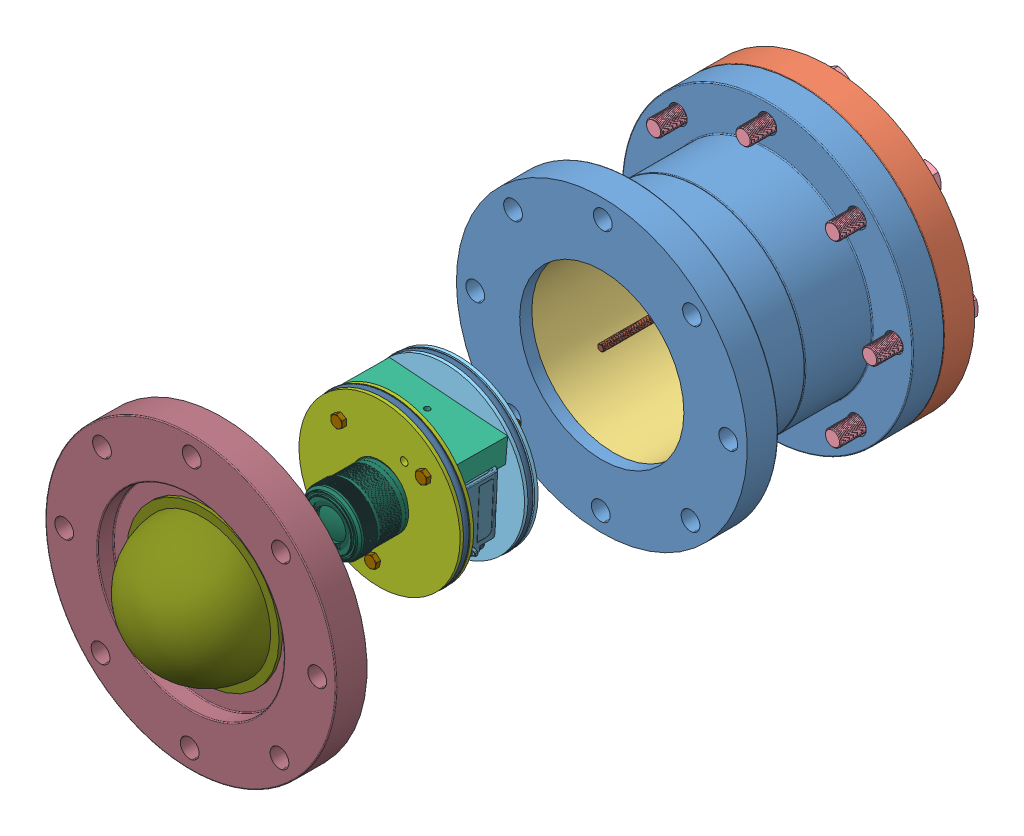
SolidWorks assembly Photogrametry_V5-PVC - exploded, configuration Default. Lengths in mm.
Overall size (484.92 484.92 825.6).
31 component instances, 16 part files, 0 mates.
Components (placement in the parent):
- externalHousing-Assembly-1: externalHousing-Assembly [Default] at (41.8532 87.3209 72.2129) size (484.92 484.92 280.15)
  - 8in PVC Flange-1: 8in PVC Flange [4881K224] at (120.5656 188.2131 202.8846) size (342.9 342.9 115.89)
  - 8in PVC Flange Closed-1: 8in PVC Flange Closed [4881K973] at (120.5656 188.2131 166.3721) size (342.9 342.9 36.51)
  - 8in PVC Pipe-1: 8in PVC Pipe [48855K43] at (120.5656 188.2131 318.8302) x (0.914978 0.403503 0) z (0 0 1) size (219.07 219.07 203.2)
  - 8in PVC Flange-2: 8in PVC Flange [4881K224] at (120.5656 188.2131 434.6169) x (-0.71277 -0.701398 0) z (0 0 -1) size (342.9 342.9 115.89)
  - BOLT 3-4in x 4in-1: BOLT 3-4in x 4in [92198A390] at (120.5656 337.4381 211.219) x (0 0 1) z (-0.999812 -0.019405 0) size (114.21 33 28.57)
  - BOLT 3-4in x 4in-2: BOLT 3-4in x 4in [92198A390] at (120.5656 38.9881 211.219) x (0 0 1) z (-0.865453 -0.50099 0) size (114.21 33 28.57)
  - BOLT 3-4in x 4in-3: BOLT 3-4in x 4in [92198A390] at (269.7906 188.2131 211.219) x (0 0 1) z (-0.997964 -0.063786 0) size (114.21 33 28.57)
  - BOLT 3-4in x 4in-4: BOLT 3-4in x 4in [92198A390] at (226.0836 82.6951 211.219) x (0 0 1) z (-0.850633 -0.525759 0) size (114.21 33 28.57)
  - BOLT 3-4in x 4in-5: BOLT 3-4in x 4in [92198A390] at (-28.6594 188.2131 211.219) x (0 0 1) z (-0.888414 -0.459043 0) size (114.21 33 28.57)
  - BOLT 3-4in x 4in-6: BOLT 3-4in x 4in [92198A390] at (15.0476 293.7311 211.219) x (0 0 1) z (-0.838585 0.544771 0) size (114.21 33 28.57)
  - BOLT 3-4in x 4in-7: BOLT 3-4in x 4in [92198A390] at (15.0476 82.6951 211.219) x (0 0 1) z (-0.991201 -0.132366 0) size (114.21 33 28.57)
  - BOLT 3-4in x 4in-8: BOLT 3-4in x 4in [92198A390] at (226.0836 293.7311 211.219) x (0 0 1) z (-0.666953 0.7451 0) size (114.21 33 28.57)
- piston-Assembly-1: piston-Assembly [Default] at (263.1271 383.964 559.12) x (-0.99718 0.075044 -0.000655) z (0 0.008727 0.999962) size (196.82 196.82 115.45)
  - piston-BackRing-1: piston-BackRing [Default] at (92.1552 117.4341 124.8546) size (190 190 16)
  - piston-CameraPlate-1: piston-CameraPlate [Default] at (92.1552 53.6841 162.8546) size (140 30 60)
  - piston-FrontRing-1: piston-FrontRing [Default] at (92.1552 117.4341 200.8546) size (190 190 16)
  - piston-SpacerTube-1: piston-SpacerTube [Default] at (92.1552 187.4341 132.8546) x (-0.829647 0.558289 0) z (0 0 1) size (18 18 60)
  - BOLT M8x110mm-1: BOLT M8x110mm [91287A317] at (42.1552 68.6841 156.5046) size (13 15.01 115.45)
  - BOLT M8x110mm-2: BOLT M8x110mm [91287A317] at (142.1552 68.6841 156.5046) x (0.995976 0.089615 0) z (0 0 1) size (13 15.01 115.45)
  - BOLT M8x110mm-3: BOLT M8x110mm [91287A317] at (92.1552 187.4341 156.5046) x (0.993023 -0.117919 0) z (0 0 1) size (13 15.01 115.45)
  - piston-7inO-RING-1: piston-7inO-RING [9452K426] at (91.7077 116.5016 200.4895) x (0.999544 -0.030202 0) z (0 0 1) size (191.13 191.13 6.99)
  - piston-7inO-RING-2: piston-7inO-RING [9452K426] at (91.7417 116.9322 125.1185) size (191.13 191.13 6.99)
- ROD M8 150mm-1: ROD M8 150mm [98861A593] at (191.0068 322.2703 396.8412) x (0 0 -1) z (1 0 0) size (281.88 8.14 9.24)
- SPRING-1: SPRING [94125K22] at (191.2399 321.4655 334.2689) x (1 0 0) z (0 0.999848 0.017452) size (11.51 82 11.48)
- 8in PVC Flange Closed - Dome Mount Cut-2: 8in PVC Flange Closed - Dome Mount Cut [4881K973] at (162.4188 275.534 955.1021) x (0.999968 -0.008041 0) z (0 0 1) size (342.9 342.9 36.51)
- A7 III + FE 28-70 v4-1: A7 III + FE 28-70 v4 [Default] at (177.6736 311.0552 735.7581) x (-0.998469 0.054614 -0.008727) z (-0.054538 -0.998474 -0.008726) size (139.07 134.7 103.31)
  - A7 III + FE 28-70 v4.step-1: A7 III + FE 28-70 v4.step [Default] at origin size (139.07 134.7 103.31)
    - Sony A7 III.step-1: Sony A7 III.step [Default] at origin size (139.07 74.69 103.31)
    - Sony FE 28-70 mm f_3.5-5.6 OSS.step-1: Sony FE 28-70 mm f_3.5-5.6 OSS.step [Default] at (13.5 -93.5 40) size (72.5 83 72.5)
- Custom Dome-1: Custom Dome [Default] at (162.4188 275.534 972.2819) x (0.91761 0.397483 0) z (0.397483 -0.91761 0) size (180 80 180)
